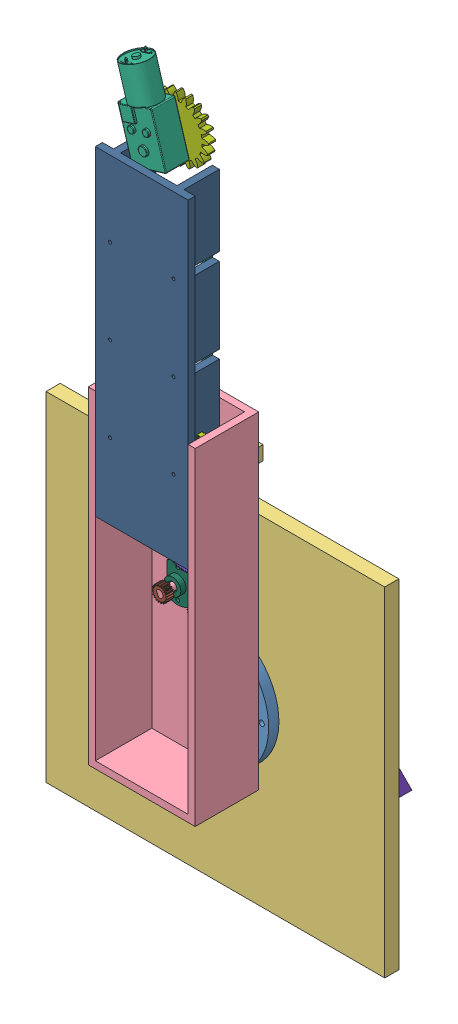
SolidWorks assembly Arm_Full_Assem_Waffle, configuration Default. Lengths in mm.
Overall size (304.8 664.74 118.61).
51 component instances, 28 part files, 103 mates.
Components (placement in the parent):
- Bearing-1: Bearing [Default] at (11.5938 121.0098 145.145) x (0 1 0) z (0 0 1) size (114.3 114.3 9.17)
  - Outside_Ring-1: Outside_Ring [Default] at (-40.6964 23.8939 0.6571) size (114.3 114.3 9.17)
  - Inside_Ring-1: Inside_Ring [Default] at (-40.6964 23.8939 0.6571) size (92.08 92.08 9.17)
- Dummy_Backplate-1: Dummy_Backplate [Default] at (-12.3001 80.3134 133.1021) size (304.8 304.8 12.7)
- Bottom_Channel-1: Bottom_Channel [Default] at (-12.3001 26.9734 161.3215) x (-1 0 0) z (0 1 0) size (96.2 57.15 294.64)
- Pancake_Motor-1: Pancake_Motor [Default] at (-16.7001 240.6134 172.9215) x (-1 0 0) z (0 0 -1) size (42 42 23.6)
- rack spur rectangular_ai-2: rack spur rectangular_ai [Inch - Rack-spur - rectangular 40DP 20PA .25FW .125PH 9L---SAll] at (-37.7001 223.8234 173.9215) x (0 1 0) z (0 0 -1) size (228.6 3.81 6.35)
- spur gear_ai-7: spur gear_ai [Inch - Spur gear 40DP 56T 20PA .25FW ---S56N3.0H2.0L0.25N] at (-16.7001 240.6134 172.9215) x (0 0 1) z (-0.791365 -0.611344 0) size (6.35 36.79 36.79)
- rack spur rectangular_ai-5: rack spur rectangular_ai [Inch - Rack-spur - rectangular 40DP 20PA .25FW .125PH 9L---SAll] at (13.0999 223.8234 180.2715) x (0 1 0) z (0 0 1) size (228.6 3.81 6.35)
- Motor_Gear-9: Motor_Gear [Default] at (-7.8101 206.1826 179.2715) x (-0.907325 0.420429 0) z (0 0 -1) size (36.82 36.82 6.35)
- Bearing_Holder-1: Bearing_Holder [Default] at (-7.8101 195.1844 161.3215) x (0 -1 0) z (-1 0 0) size (24.67 10.16 41.05)
- Inside_Channel-1: Inside_Channel [Default] at (-44.0501 512.1134 174.0215) x (1 0 0) z (0 -1 0) size (83.5 38.1 288.29)
- Pancake_Motor-2: Pancake_Motor [Default] at (-12.3001 491.1134 194.1715) size (42 42 23.6) (hidden)
- spur gear_ai-11: spur gear_ai [Inch - Spur gear 10DP 20T 20PA 0.25FW ---S20N3.0H2.0L0.25N] at (-16.584 526.2798 169.2715) x (0 0 1) z (-0.088369 -0.996088 0) size (6.35 55.38 55.38)
- Idler_Gear-12: Idler_Gear [Default] at (-28.1751 160.3234 180.2715) x (0.915999 0.401182 0) z (0 0 -1) size (13.95 13.95 6.35)
- Idler_Gear-13: Idler_Gear [Default] at (3.5749 160.3234 180.2715) x (0.910058 -0.414481 0) z (0 0 -1) size (13.95 13.95 6.35)
- Slip_Ring-1: Slip_Ring [Default] at (-12.3001 80.3134 121.1771) x (-0.506377 -0.862312 0) z (0 0 1) size (44 44 39.4)
- spur gear_ai-15: spur gear_ai [Inch - Spur gear 10DP 40T 20PA .25FW ---S40N3.0H2.0L0.25N] at (59.542 8.4713 129.9271) x (0 0 -1) z (0.885459 0.464717 0) size (6.35 106.46 106.46)
- Encoder-1: Encoder [Default] at (45.4422 5.6005 93.5071) x (0.707107 -0.707107 0) z (0 0 1) size (15.88 21.21 36.42)
- spur gear_ai-16: spur gear_ai [Inch - Spur gear 10DP 40T 20PA .25FW ---S40N3.0H2.0L0.5N] at (-84.1421 152.1554 129.9271) x (0 0 -1) z (-0.884026 -0.467439 0) size (6.35 106.46 106.46)
- Coupling-1: Coupling [Default] at (-16.584 526.2798 175.6215) x (0.44043 -0.897787 0) z (0 0 1) size (12.7 12.7 25.4) (hidden)
- Gear_Shaft-1: Gear_Shaft [Default] at (-16.584 526.2798 188.3215) x (-0.201369 0.979515 0) z (0 0 -1) size (6.35 6.35 19.05) (hidden)
- Center_Gear-1: Center_Gear [Default] at (-12.3001 80.3134 123.5771) x (-0.493596 0.869691 0) z (0 0 1) size (106.51 106.51 6.35)
- Small_Bearing_Holder-1: Small_Bearing_Holder [Default] at (-44.8751 160.3234 161.3215) x (-1 0 0) z (0 0 -1) size (19.05 33.4 7.3)
- Small_Bearing_Holder-2: Small_Bearing_Holder [Default] at (-13.1251 160.3234 161.3215) x (-1 0 0) z (0 0 -1) size (19.05 33.4 7.3)
- 10mm_Bearing-2: 10mm_Bearing [7804K1] at (3.5749 160.3234 163.3215) x (0.99661 0.082273 0) z (0 0 1) size (10 10 4)
- Encoder_Holder-1: Encoder_Holder [Default] at (0.1843 -23.9456 104.5271) x (0.707107 0.707107 0) z (0 0 -1) size (152.4 38.1 34.92)
- 5_16_Bearing-3: 5_16_Bearing [60355K503] at (-84.1421 152.1554 140.2459) x (-0.2744 -0.961616 0) z (0 0 1) size (15.88 15.88 4.76)
- 5_16_Bearing-5: 5_16_Bearing [60355K503] at (59.542 8.4713 140.2459) size (15.88 15.88 4.76)
- Graphite_Brush-1: Graphite_Brush [Default] at (22.568 289.9752 170.3294) x (1 0 0) z (0 0 -1) size (5.52 5.52 23.23)
  - Graphite-1: Graphite [Default] at (0.6919 3.2868 2.6579) size (5.08 5.08 10.16)
  - Graphite_Spring-1: Graphite_Spring [9657K268] at (3.2319 5.8268 25.5179) size (5.52 5.52 13.07)
- Graphite_Brush-2: Graphite_Brush [Default] at (13.043 289.9752 170.3294) x (1 0 0) z (0 0 -1) size (5.52 5.52 23.23)
  - Graphite-1: Graphite [Default] at (0.6919 3.2868 2.6579) size (5.08 5.08 10.16)
  - Graphite_Spring-1: Graphite_Spring [9657K268] at (3.2319 5.8268 25.5179) size (5.52 5.52 13.07)
- Graphite_Brush-3: Graphite_Brush [Default] at (-37.6431 278.3216 170.3294) x (-1 0 0) z (0 0 -1) size (5.52 5.52 23.23)
  - Graphite-1: Graphite [Default] at (0.6919 3.2868 2.6579) size (5.08 5.08 10.16)
  - Graphite_Spring-1: Graphite_Spring [9657K268] at (3.2319 5.8268 25.5179) size (5.52 5.52 13.07)
- Graphite_Brush-4: Graphite_Brush [Default] at (-47.1681 278.3216 170.3294) x (-1 0 0) z (0 0 -1) size (5.52 5.52 23.23)
  - Graphite-1: Graphite [Default] at (0.6919 3.2868 2.6579) size (5.08 5.08 10.16)
  - Graphite_Spring-1: Graphite_Spring [9657K268] at (3.2319 5.8268 25.5179) size (5.52 5.52 13.07)
- Brush_Holder-1: Brush_Holder [Default] at (9.9249 284.1484 147.3515) x (0 1 0) z (1 0 0) size (25.4 7.62 22.23)
- Brush_Holder-2: Brush_Holder [Default] at (-56.7501 284.1484 147.3515) x (0 1 0) z (1 0 0) size (25.4 7.62 22.23)
- Small_Gear_Shaft-1: Small_Gear_Shaft [Default] at (-28.1751 160.3234 166.2715) x (0.915999 0.401182 0) z (0 0 1) size (6.35 6.35 14)
- Small_Gear_Shaft-2: Small_Gear_Shaft [Default] at (3.5749 160.3234 166.2715) x (0.910058 -0.414481 0) z (0 0 1) size (6.35 6.35 14)
- Small_Gear_Shaft-3: Small_Gear_Shaft [Large_Gear] at (-7.8101 206.1826 165.2715) x (0.907325 -0.420429 0) z (0 0 1) size (10 10 10.95)
- 10mm_Bearing-3: 10mm_Bearing [7804K1] at (-28.1751 160.3234 163.3215) x (0.999767 0.021604 0) z (0 0 1) size (10 10 4)
- 22mm_Bearing-1: 22mm_Bearing [5972K91] at (-7.8101 206.1826 164.8215) x (0.980177 0.198125 0) z (0 0 1) size (22 22 7)
- 1P0000_BrushMotor-1: 1P0000_BrushMotor [Default] at (-10.0974 560.1055 184.2715) x (0.289457 -0.957191 0) z (0.957191 0.289457 0) size (80 40 32)
- Linear_Guide_Rail-1: Linear_Guide_Rail [6725K28] at (29.4499 33.3234 198.2715) x (0 1 0) z (0 0 1) size (288.29 3.7 5)
- Linear_Guide_Carriage-1: Linear_Guide_Carriage [6725K1] at (29.4499 50.4945 198.2715) x (0 0 1) z (0 -1 0) size (12 5 19)
Mates (geometry in assembly coordinates):
- Coincident1: coincident: plane of Bearing-1/Outside_Ring-1 through (-12.3001 80.3134 145.8021) normal (0 0 -1); plane of Dummy_Backplate-1 through (-12.3001 80.3134 145.8021) normal (0 0 1)
- Concentric1: concentric: circle of Bearing-1/Inside_Ring-1; circle of Dummy_Backplate-1
- Concentric2: concentric: circle of Bearing-1/Inside_Ring-1; circle of Bottom_Channel-1
- Concentric3: concentric: circle of Bearing-1/Inside_Ring-1; circle of Bottom_Channel-1
- Coincident4: coincident: plane of Bearing-1/Inside_Ring-1 through (-12.3001 80.3134 154.9715) normal (0 0 1); plane of Bottom_Channel-1 through (-60.4001 321.6134 154.9715) normal (0 0 -1)
- Coincident5: coincident: plane of Bottom_Channel-1 through (-12.3001 321.6134 161.3215) normal (0 0 1); plane of Pancake_Motor-1 through (-16.7001 240.6134 161.3215) normal (0 0 -1)
- Distance1: distance = 60 mm: plane of Pancake_Motor-1 through (-37.7001 261.6134 161.3215) normal (0 1 0); plane of Bottom_Channel-1 through (-12.3001 321.6134 161.3215) normal (0 1 0)
- Distance6: distance = 16.35 mm: plane of Bottom_Channel-1 through (-54.0501 321.6134 183.5465) normal (1 0 0); plane of Pancake_Motor-1 through (-37.7001 261.6134 161.3215) normal (-1 0 0)
- Distance3: distance = 1 mm: plane of rack spur rectangular_ai-2 through (-33.8901 223.8234 173.9215) normal (0 0 -1); plane of Pancake_Motor-1 through (-16.7001 240.6134 172.9215) normal (0 0 1)
- Coincident13: coincident: plane of Pancake_Motor-1 through (-16.7001 240.6134 172.9215) normal (0 0 1); plane of spur gear_ai-7 through (-16.7001 240.6134 172.9215) normal (0 0 -1)
- Concentric6: concentric: circle of Pancake_Motor-1; cylinder of spur gear_ai-7 through (-16.7001 240.6134 223.7216) axis (0 0 -1) radius 3.175
- Coincident54: coincident: plane of rack spur rectangular_ai-5 through (13.0999 223.8234 173.9215) normal (1 0 0); plane of Inside_Channel-1 through (13.0999 223.8234 174.0215) normal (-1 0 0)
- Distance11: distance = 1 mm: plane of Pancake_Motor-1 through (-16.7001 240.6134 172.9215) normal (0 0 1); plane of rack spur rectangular_ai-5 through (9.2899 223.8234 173.9215) normal (0 0 -1)
- Coincident17: coincident: plane of rack spur rectangular_ai-2 through (-37.7001 452.4234 180.2715) normal (0 1 0); plane of rack spur rectangular_ai-5 through (13.0999 452.4234 173.9215) normal (0 1 0)
- Concentric8: concentric: circle of Bottom_Channel-1; circle of Bearing_Holder-1
- Coincident20: coincident: plane of Bottom_Channel-1 through (-12.3001 321.6134 161.3215) normal (0 0 1); plane of Bearing_Holder-1 through (-7.8101 195.1844 161.3215) normal (0 0 -1)
- RackPinionMate1: rack pinion = 35.56 mm: line of rack spur rectangular_ai-2 through (-37.7001 223.8234 180.2715) axis (0 1 0); circle of spur gear_ai-7
- Distance16: distance = 10 mm: plane of Bottom_Channel-1 through (29.4499 321.6134 183.5465) normal (-1 0 0); plane of Inside_Channel-1 through (19.4499 223.8234 183.5465) normal (1 0 0)
- Coincident23: coincident: plane of rack spur rectangular_ai-5 through (13.0999 223.8234 173.9215) normal (0 -1 0); plane of Inside_Channel-1 through (-44.0501 223.8234 174.0215) normal (0 -1 0)
- LimitDistance1: limit distance = 190.5 mm: plane of Inside_Channel-1 through (-44.0501 223.8234 174.0215) normal (0 -1 0); plane of Bottom_Channel-1 through (-54.0501 33.3234 295.8626) normal (0 1 0)
- Coincident24: coincident: plane of Inside_Channel-1 through (-37.7001 223.8234 205.7715) normal (0 0 -1); plane of Pancake_Motor-2 through (-12.3001 491.1134 205.7715) normal (0 0 1)
- Width1: width: plane of Bottom_Channel-1 through (29.4499 321.6134 183.5465) normal (-1 0 0); plane of Bottom_Channel-1 through (-54.0501 321.6134 183.5465) normal (1 0 0); plane of Pancake_Motor-2 through (8.6999 512.1134 205.7715) normal (1 0 0); plane of Pancake_Motor-2 through (-33.3001 512.1134 205.7715) normal (-1 0 0)
- Coincident25: coincident: line of Inside_Channel-1 through (-37.7001 512.1134 205.7715) axis (1 0 0); line of Pancake_Motor-2 through (8.6999 512.1134 205.7715) axis (-1 0 0)
- Concentric9: concentric: circle of Pancake_Motor-2; circle of spur gear_ai-11
- Distance8: distance = 22.86 mm: plane of spur gear_ai-11 through (-16.584 526.2798 175.6215) normal (0 0 1); plane of Dummy_Backplate-1 through (-12.3001 80.3134 145.8021) normal (0 0 1)
- Parallel1: parallel: plane of Bottom_Channel-1 through (35.7999 321.6134 212.1215) normal (1 0 0); plane of assembly through (0 0 0) normal (1 0 0)
- Distance13: distance = 3.175 mm: plane of spur gear_ai-15 through (59.542 8.4713 129.9271) normal (0 0 1); plane of Dummy_Backplate-1 through (-12.3001 80.3134 133.1021) normal (0 0 -1)
- Concentric14: concentric: circle of spur gear_ai-15; circle of Encoder-1
- Coincident30: coincident: plane of spur gear_ai-15 through (59.542 8.4713 129.9271) normal (0 0 1); plane of Encoder-1 through (45.4422 5.6005 129.9271) normal (0 0 1)
- Concentric15: concentric: circle of spur gear_ai-15; circle of Dummy_Backplate-1
- Concentric16: concentric: circle of spur gear_ai-16; cylinder of Dummy_Backplate-1 through (-84.1421 152.1554 168.2527) axis (0 0 -1) radius 7.9375
- Distance14: distance = 3.175 mm: plane of spur gear_ai-16 through (-84.1421 152.1554 129.9271) normal (0 0 1); plane of Dummy_Backplate-1 through (-12.3001 80.3134 133.1021) normal (0 0 -1)
- Concentric17: concentric: circle of Pancake_Motor-2; circle of Coupling-1
- Coincident32: coincident: plane of Pancake_Motor-2 through (-12.3001 300.6134 194.1715) normal (0 0 -1); plane of Coupling-1 through (-12.3001 300.6134 194.1715) normal (0 0 1)
- Concentric18: concentric: circle of spur gear_ai-11; circle of Gear_Shaft-1
- Coincident34: coincident: plane of Coupling-1 through (-16.584 526.2798 188.3215) normal (0 0 -1); plane of Gear_Shaft-1 through (-16.584 526.2798 188.3215) normal (0 0 1)
- Distance15: distance = 3.175 mm: plane of Center_Gear-1 through (-10.6229 56.5042 129.9271) normal (0 0 1); plane of Dummy_Backplate-1 through (-12.3001 80.3134 133.1021) normal (0 0 -1)
- Concentric19: concentric: circle of Bearing-1/Outside_Ring-1; circle of Center_Gear-1
- Concentric20: concentric: circle of Bearing-1/Inside_Ring-1; circle of Center_Gear-1
- Concentric21: concentric: circle of Slip_Ring-1; circle of Center_Gear-1
- Concentric22: concentric: circle of Slip_Ring-1; circle of Center_Gear-1
- Coincident39: coincident: plane of Slip_Ring-1 through (-12.3001 80.3134 123.5771) normal (0 0 1); plane of Center_Gear-1 through (-10.6229 56.5042 123.5771) normal (0 0 -1)
- GearMate2: gear = 60.3225 : 95.2475 mm: circle of Center_Gear-1; circle of spur gear_ai-15
- GearMate3: gear = 95.2475 : 60.3225 mm: circle of spur gear_ai-16; circle of Center_Gear-1
- Coincident40: coincident: plane of Bottom_Channel-1 through (-54.0501 321.6134 212.1215) normal (0 0 1); plane of Inside_Channel-1 through (-44.0501 223.8234 212.1215) normal (0 0 1)
- Parallel2: parallel: plane of Pancake_Motor-1 through (-37.7001 219.6134 161.3215) normal (0 -1 0); plane of Bearing_Holder-1 through (9.3584 218.4508 124.7233) normal (0 1 0)
- Coincident43: coincident: plane of Bottom_Channel-1 through (-12.3001 321.6134 161.3215) normal (0 0 1); plane of Small_Bearing_Holder-1 through (-44.8751 160.3234 161.3215) normal (0 0 -1)
- Parallel3: parallel: plane of Bottom_Channel-1 through (-54.0501 321.6134 183.5465) normal (1 0 0); plane of Small_Bearing_Holder-1 through (-18.6501 144.4484 120.6617) normal (1 0 0)
- Coincident45: coincident: plane of Bottom_Channel-1 through (-12.3001 321.6134 161.3215) normal (0 0 1); plane of Small_Bearing_Holder-2 through (-13.1251 160.3234 161.3215) normal (0 0 -1)
- Concentric25: concentric: cylinder of Bottom_Channel-1 through (3.5749 160.3234 212.1215) axis (0 0 -1) radius 3.175; circle of Small_Bearing_Holder-2
- Parallel4: parallel: plane of Bottom_Channel-1 through (29.4499 321.6134 183.5465) normal (-1 0 0); plane of Small_Bearing_Holder-2 through (-5.9501 144.4484 120.6617) normal (-1 0 0)
- Concentric26: concentric: circle of Small_Bearing_Holder-2; circle of 10mm_Bearing-2
- Coincident47: coincident: plane of Bottom_Channel-1 through (-12.3001 321.6134 161.3215) normal (0 0 1); plane of 10mm_Bearing-2 through (3.18 165.1071 161.3215) normal (0 0 -1)
- Coincident48: coincident: plane of Dummy_Backplate-1 through (-12.3001 80.3134 133.1021) normal (0 0 -1); plane of Encoder_Holder-1 through (0.1843 -23.9456 133.1021) normal (0 0 1)
- Coincident49: coincident: plane of Encoder-1 through (45.4422 5.6005 107.3971) normal (-0.707107 0.707107 0); plane of Encoder_Holder-1 through (45.443 5.6012 98.1771) normal (0.707107 -0.707107 0)
- Coincident50: coincident: plane of Encoder-1 through (60.44 20.5982 107.3971) normal (0.707107 0.707107 0); plane of Encoder_Holder-1 through (60.44 20.5982 98.1771) normal (-0.707107 -0.707107 0)
- Angle1: planar angle = 0.785398 rad: plane of Dummy_Backplate-1 through (140.0999 -72.0866 145.8021) normal (0 -1 0); plane of Encoder_Holder-1 through (27.125 -50.8864 98.1771) normal (0.707107 -0.707107 0)
- Concentric27: concentric: circle of Dummy_Backplate-1; circle of 5_16_Bearing-3
- Coincident51: coincident: plane of Dummy_Backplate-1 through (-12.3001 80.3134 142.6271) normal (0 0 -1); plane of 5_16_Bearing-3 through (-76.7383 150.0427 142.6271) normal (0 0 1)
- Concentric28: concentric: circle of Dummy_Backplate-1; circle of 5_16_Bearing-5
- Coincident53: coincident: plane of Dummy_Backplate-1 through (-12.3001 80.3134 142.6271) normal (0 0 -1); plane of 5_16_Bearing-5 through (59.542 16.1707 142.6271) normal (0 0 1)
- Coincident56: coincident: plane of rack spur rectangular_ai-2 through (-37.7001 223.8234 180.2715) normal (-1 0 0); plane of Inside_Channel-1 through (-37.7001 223.8234 174.0215) normal (1 0 0)
- Width3: width: plane of Bottom_Channel-1 through (22.6249 287.3234 145.9913) normal (1 0 0); plane of Bottom_Channel-1 through (28.9749 287.3234 145.9913) normal (-1 0 0); plane of Graphite_Brush-1/Graphite-1 through (28.3399 286.6884 157.5115) normal (1 0 0); plane of Graphite_Brush-1/Graphite-1 through (23.2599 286.6884 157.5115) normal (-1 0 0)
- Width4: width: plane of Bottom_Channel-1 through (28.9749 287.3234 145.9913) normal (-1 0 0); plane of Bottom_Channel-1 through (22.6249 287.3234 145.9913) normal (1 0 0); plane of Graphite_Brush-1/Graphite-1 through (28.3399 286.6884 157.5115) normal (1 0 0); plane of Graphite_Brush-1/Graphite-1 through (23.2599 286.6884 157.5115) normal (-1 0 0)
- Width5: width: plane of Bottom_Channel-1 through (22.6249 280.9734 145.9913) normal (0 1 0); plane of Bottom_Channel-1 through (22.6249 287.3234 145.9913) normal (0 -1 0); plane of Graphite_Brush-1/Graphite-1 through (23.2599 286.6884 157.5115) normal (0 1 0); plane of Graphite_Brush-1/Graphite-1 through (23.2599 281.6084 157.5115) normal (0 -1 0)
- Coincident85: coincident: line of Bottom_Channel-1 through (28.9749 287.3234 154.9715) axis (-1 0 0); line of Brush_Holder-1 through (22.6249 287.3234 154.9715) axis (1 0 0)
- Coincident86: coincident: plane of Bottom_Channel-1 through (-60.4001 321.6134 154.9715) normal (0 0 -1); plane of Brush_Holder-1 through (21.0374 284.1484 154.9715) normal (0 0 1)
- Coincident87: coincident: line of Bottom_Channel-1 through (28.9749 280.9734 154.9715) axis (0 1 0); line of Brush_Holder-1 through (28.9749 287.3234 154.9715) axis (0 -1 0)
- Concentric32: concentric: circle of Small_Bearing_Holder-1; circle of 10mm_Bearing-3
- Coincident94: coincident: plane of Bottom_Channel-1 through (-12.3001 321.6134 161.3215) normal (0 0 1); plane of 10mm_Bearing-3 through (-28.2788 165.1223 161.3215) normal (0 0 -1)
- Concentric33: concentric: circle of Bottom_Channel-1; circle of Small_Bearing_Holder-1
- Concentric34: concentric: circle of Bottom_Channel-1; circle of 22mm_Bearing-1
- Coincident95: coincident: plane of Bottom_Channel-1 through (-12.3001 321.6134 161.3215) normal (0 0 1); plane of 22mm_Bearing-1 through (-9.9201 216.6214 161.3215) normal (0 0 -1)
- Concentric35: concentric: circle of Motor_Gear-9; circle of 22mm_Bearing-1
- Coincident97: coincident: plane of Motor_Gear-9 through (-7.8101 206.1826 179.2715) normal (0 0 1); plane of Small_Gear_Shaft-3 through (-7.8101 206.1826 179.2715) normal (0 0 1)
- Coincident99: coincident: plane of Motor_Gear-9 through (-7.8101 206.1826 179.2715) normal (0 0 1); plane of spur gear_ai-7 through (-16.7001 240.6134 179.2715) normal (0 0 1)
- Concentric36: concentric: unknown of Motor_Gear-9; unknown of Small_Gear_Shaft-3
- GearMate4: gear = 33.9344 : 33.9344 mm: circle of Motor_Gear-9; circle of spur gear_ai-7
- Coincident100: coincident: line of Motor_Gear-9 through (-10.6064 204.6789 179.2715) axis (0.420429 0.907325 0); line of Small_Gear_Shaft-3 through (-10.6064 204.6789 179.2715) axis (0.420429 0.907325 0)
- Concentric37: concentric: circle of Idler_Gear-12; circle of Small_Gear_Shaft-1
- Concentric38: concentric: circle of Small_Gear_Shaft-1; circle of 10mm_Bearing-3
- Coincident102: coincident: plane of Idler_Gear-12 through (-25.2509 160.9156 180.2715) normal (0 0 1); plane of Small_Gear_Shaft-1 through (-28.1751 160.3234 180.2715) normal (0 0 1)
- Coincident103: coincident: plane of rack spur rectangular_ai-2 through (-33.8901 223.8234 180.2715) normal (0 0 1); plane of Idler_Gear-12 through (-25.2509 160.9156 180.2715) normal (0 0 1)
- Coincident104: coincident: line of Idler_Gear-12 through (-28.9011 157.2325 180.2715) axis (-0.401182 0.915999 0); line of Small_Gear_Shaft-1 through (-28.9011 157.2325 180.2715) axis (-0.401182 0.915999 0)
- RackPinionMate3: rack pinion = 11.0744 mm: line of rack spur rectangular_ai-2 through (-37.7001 223.8234 180.2715) axis (0 1 0); circle of Idler_Gear-12
- Concentric39: concentric: circle of 10mm_Bearing-2; circle of Small_Gear_Shaft-2
- Concentric40: concentric: circle of Idler_Gear-13; circle of Small_Gear_Shaft-2
- Coincident107: coincident: plane of Idler_Gear-13 through (5.9673 158.5407 180.2715) normal (0 0 1); plane of Small_Gear_Shaft-2 through (3.5749 160.3234 180.2715) normal (0 0 1)
- Coincident108: coincident: plane of rack spur rectangular_ai-5 through (9.2899 223.8234 180.2715) normal (0 0 1); plane of Idler_Gear-13 through (5.9673 158.5407 180.2715) normal (0 0 1)
- Coincident109: coincident: line of Idler_Gear-13 through (0.7885 158.8014 180.2715) axis (0.414481 0.910058 0); line of Small_Gear_Shaft-2 through (0.7885 158.8014 180.2715) axis (0.414481 0.910058 0)
- RackPinionMate4: rack pinion = 11.0744 mm: line of rack spur rectangular_ai-5 through (13.0999 223.8234 180.2715) axis (0 1 0); circle of Idler_Gear-13
- Coincident111: coincident: plane of Inside_Channel-1 through (-37.7001 223.8234 205.7715) normal (0 0 -1); plane of 1P0000_BrushMotor-1 through (-10.0974 560.1055 205.7715) normal (0 0 1)
- Coincident115: coincident: moEndPointRef_w of Inside_Channel-1; unknown of 1P0000_BrushMotor-1
- Coincident116: coincident: plane of spur gear_ai-11 through (-16.584 526.2798 169.2715) normal (0 0 -1); plane of Gear_Shaft-1 through (-16.584 526.2798 169.2715) normal (0 0 -1)
- Concentric41: concentric: circle of Coupling-1; circle of Gear_Shaft-1
- Concentric42: concentric: circle of spur gear_ai-11; circle of 1P0000_BrushMotor-1
- Coincident118: coincident: plane of spur gear_ai-11 through (-16.584 526.2798 169.2715) normal (0 0 -1); plane of 1P0000_BrushMotor-1 through (-10.0974 560.1055 169.2715) normal (0 0 -1)
- Coincident119: coincident: plane of Bottom_Channel-1 through (29.4499 321.6134 183.5465) normal (-1 0 0); plane of Linear_Guide_Rail-1 through (29.4499 321.6134 195.4715) normal (1 0 0)
- Coincident120: coincident: plane of Bottom_Channel-1 through (-12.3001 321.6134 161.3215) normal (0 1 0); plane of Linear_Guide_Rail-1 through (27.2499 321.6134 190.6215) normal (0 1 0)
- Distance17: distance = 11.35 mm: plane of Linear_Guide_Rail-1 through (27.7269 321.6134 200.7715) normal (0 0 1); plane of Bottom_Channel-1 through (-54.0501 321.6134 212.1215) normal (0 0 1)
- Coincident122: coincident: plane of Linear_Guide_Rail-1 through (26.7729 321.6134 190.7715) normal (0 0 -1); plane of Linear_Guide_Carriage-1 through (26.1499 40.9945 190.7715) normal (0 0 1)
- Coincident123: coincident: plane of Linear_Guide_Rail-1 through (25.7499 321.6134 191.0715) normal (-1 0 0); plane of Linear_Guide_Carriage-1 through (25.7499 40.9945 195.4715) normal (1 0 0)
- LimitDistance2: limit distance = 261.6188 mm: plane of Linear_Guide_Carriage-1 through (25.9499 59.9945 190.4215) normal (0 1 0); plane of Linear_Guide_Rail-1 through (27.2499 321.6134 195.6215) normal (0 1 0)
